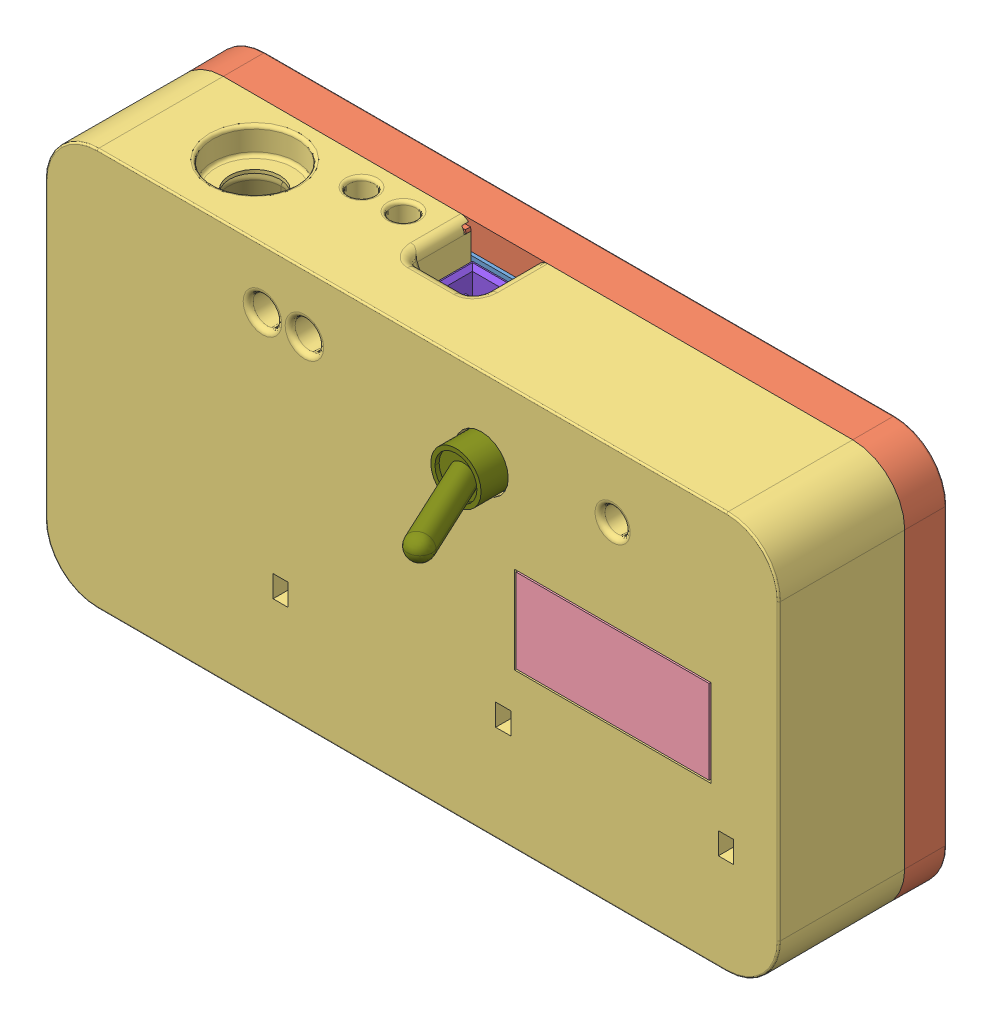
SolidWorks assembly index, configuration 默认. Lengths in mm.
Overall size (87.4 47.4 33.7).
302 component instances, 40 part files, 15 mates.
Components (placement in the parent):
- PowerSupplyBoard-1: PowerSupplyBoard [默认] at origin size (80 40 32.5)
  - PCB2.step-1: PCB2.step [默认] at origin size (80 40 32.5)
    - Board.step-1: Board.step [默认] at origin size (80 40 1.6)
      - Open CASCADE STEP translator 6.8 2.1.1.step-1: Open CASCADE STEP translator 6.8 2.1.1.step [默认] at (0 0 -1.6) size (80 40 1.6)
    - C1.step-1: C1.step [默认] at origin size (0.82 1.6 0.82)
      - C_0603.step-1: C_0603.step [默认] at (74.2189 27.7979 0.0254) x (0 -1 0) z (0 0 1) size (1.6 0.82 0.82)
        - C_0603-7177_AF0_ASM.step-1: C_0603-7177_AF0_ASM.step [默认] at origin size (1.6 0.82 0.82)
          - C_0603-683_AF0_ASM.step-1: C_0603-683_AF0_ASM.step [默认] at origin size (1.6 0.82 0.82)
            - 2_1_200.step-1: 2_1_200.step [默认] at origin size (0.3 0.82 0.82)
            - _1_1_20001.step-1: _1_1_20001.step [默认] at origin size (1 0.8 0.8)
            - 3_1_2_A.step-1: 3_1_2_A.step [默认] at origin size (0.3 0.82 0.82)
    - C3.step-1: C3.step [默认] at origin size (7 6.6 5.41)
      - CM_D(6.3X5.4).step-1: CM_D(6.3X5.4).step [默认] at (74.7014 21.0058 0) x (0 1 0) z (0 0 1) size (6.6 7 5.41)
        - LOGO_.step-1: LOGO_.step [默认] at (1.6383 0.2015 -0.0035) x (-1 0 0) z (0 0 -1) size (1.35 1.56 0.01)
        - CM_D(6.3X5.4)-0.step-1: CM_D(6.3X5.4)-0.step [默认] at origin size (6.6 7 5.41)
    - Open CASCADE STEP translator 6.8 2.4.step-1: Open CASCADE STEP translator 6.8 2.4.step [默认] at origin size (7.54 7.7 9.1)
      - XH2.54-2P_H.step-1: XH2.54-2P_H.step [默认] at (37.2618 32.1564 0.03) x (-1 0 0) z (0 1 0) size (7.54 9.1 7.7)
        - LOGO_-1.step-1: LOGO_-1.step [默认] at (-1.159 -0.003 2.4494) x (0 0 1) z (0 -1 0) size (0.9 1.04 0.01)
        - XH2.54-2P_H-2.step-1: XH2.54-2P_H-2.step [默认] at origin size (7.54 9.1 7.7)
    - Open CASCADE STEP translator 6.8 2.5.step-1: Open CASCADE STEP translator 6.8 2.5.step [默认] at origin size (10.16 12.85 8.1)
      - HDR-1x2_H.step-1: HDR-1x2_H.step [默认] at (40.6527 12.7 0) x (1 0 0) z (0 0 1) size (2.54 12.85 8.1)
        - HDR-1x2_H-3.step-1: HDR-1x2_H-3.step [默认] at origin size (2.54 12.85 8.1)
        - LOGO_-4.step-1: LOGO_-4.step [默认] at (0 -4.7829 0.017) x (-1 0 0) z (0 0 -1) size (0.9 1.04 0.01)
      - HDR-1x2_H.step-2: HDR-1x2_H.step [默认] at (43.1927 12.7 0) x (1 0 0) z (0 0 1) size (2.54 12.85 8.1)
        - HDR-1x2_H-3.step-1: HDR-1x2_H-3.step [默认] at origin size (2.54 12.85 8.1)
        - LOGO_-4.step-1: LOGO_-4.step [默认] at (0 -4.7829 0.017) x (-1 0 0) z (0 0 -1) size (0.9 1.04 0.01)
      - HDR-1x2_H.step-3: HDR-1x2_H.step [默认] at (35.5727 12.7 0) x (1 0 0) z (0 0 1) size (2.54 12.85 8.1)
        - HDR-1x2_H-3.step-1: HDR-1x2_H-3.step [默认] at origin size (2.54 12.85 8.1)
        - LOGO_-4.step-1: LOGO_-4.step [默认] at (0 -4.7829 0.017) x (-1 0 0) z (0 0 -1) size (0.9 1.04 0.01)
      - HDR-1x2_H.step-4: HDR-1x2_H.step [默认] at (38.1127 12.7 0) x (1 0 0) z (0 0 1) size (2.54 12.85 8.1)
        - HDR-1x2_H-3.step-1: HDR-1x2_H-3.step [默认] at origin size (2.54 12.85 8.1)
        - LOGO_-4.step-1: LOGO_-4.step [默认] at (0 -4.7829 0.017) x (-1 0 0) z (0 0 -1) size (0.9 1.04 0.01)
    - Open CASCADE STEP translator 6.8 2.6.step-1: Open CASCADE STEP translator 6.8 2.6.step [默认] at origin size (5 6.01 1.9)
      - SOP8.step-1: SOP8.step [默认] at (39.878 26.6954 0) x (0 1 0) z (0 0 1) size (6.01 5 1.9)
        - LOGO_0.25.step-1: LOGO_0.25.step [默认] at (0.0116 0 0.095) x (0 -1 0) z (0 0 -1) size (0.75 0.87 0.01)
        - SOP8_____.step-1: SOP8_____.step [默认] at origin size (3.6 5 1.8)
        - ____1.8_______.step-1: ____1.8_______.step [默认] at (1.8 1.91 1) x (0 1 0) z (0 0 1) size (0.5 1.2 1.1)
        - ____1.8_______.step-2: ____1.8_______.step [默认] at (1.8 0.64 1) x (0 1 0) z (0 0 1) size (0.5 1.2 1.1)
        - ____1.8_______.step-3: ____1.8_______.step [默认] at (1.8 -0.63 1) x (0 1 0) z (0 0 1) size (0.5 1.2 1.1)
        - ____1.8_______.step-4: ____1.8_______.step [默认] at (1.8 -1.9 1) x (0 1 0) z (0 0 1) size (0.5 1.2 1.1)
        - ____1.8_______.step-5: ____1.8_______.step [默认] at (-1.8 1.91 1) x (0 -1 0) z (0 0 1) size (0.5 1.2 1.1)
        - ____1.8_______.step-6: ____1.8_______.step [默认] at (-1.8 0.64 1) x (0 -1 0) z (0 0 1) size (0.5 1.2 1.1)
        - ____1.8_______.step-7: ____1.8_______.step [默认] at (-1.8 -0.63 1) x (0 -1 0) z (0 0 1) size (0.5 1.2 1.1)
        - ____1.8_______.step-8: ____1.8_______.step [默认] at (-1.8 -1.9 1) x (0 -1 0) z (0 0 1) size (0.5 1.2 1.1)
    - Open CASCADE STEP translator 6.8 2.7.step-1: Open CASCADE STEP translator 6.8 2.7.step [默认] at origin size (5 6.01 1.9)
      - SOP8.step-1: SOP8.step [默认] at (66.9036 26.6954 0) x (0 1 0) z (0 0 1) size (6.01 5 1.9)
        - LOGO_0.25.step-1: LOGO_0.25.step [默认] at (0.0116 0 0.095) x (0 -1 0) z (0 0 -1) size (0.75 0.87 0.01)
        - SOP8_____.step-1: SOP8_____.step [默认] at origin size (3.6 5 1.8)
        - ____1.8_______.step-1: ____1.8_______.step [默认] at (1.8 1.91 1) x (0 1 0) z (0 0 1) size (0.5 1.2 1.1)
        - ____1.8_______.step-2: ____1.8_______.step [默认] at (1.8 0.64 1) x (0 1 0) z (0 0 1) size (0.5 1.2 1.1)
        - ____1.8_______.step-3: ____1.8_______.step [默认] at (1.8 -0.63 1) x (0 1 0) z (0 0 1) size (0.5 1.2 1.1)
        - ____1.8_______.step-4: ____1.8_______.step [默认] at (1.8 -1.9 1) x (0 1 0) z (0 0 1) size (0.5 1.2 1.1)
        - ____1.8_______.step-5: ____1.8_______.step [默认] at (-1.8 1.91 1) x (0 -1 0) z (0 0 1) size (0.5 1.2 1.1)
        - ____1.8_______.step-6: ____1.8_______.step [默认] at (-1.8 0.64 1) x (0 -1 0) z (0 0 1) size (0.5 1.2 1.1)
        - ____1.8_______.step-7: ____1.8_______.step [默认] at (-1.8 -0.63 1) x (0 -1 0) z (0 0 1) size (0.5 1.2 1.1)
        - ____1.8_______.step-8: ____1.8_______.step [默认] at (-1.8 -1.9 1) x (0 -1 0) z (0 0 1) size (0.5 1.2 1.1)
    - R6.step-1: R6.step [默认] at origin size (0.8 1.6 0.4)
      - R0603.step-1: R0603.step [默认] at (44.6277 27.5996 0) x (0 1 0) z (0 0 1) size (1.6 0.8 0.4)
        - R_0603-3615_AF0_ASM.step-1: R_0603-3615_AF0_ASM.step [默认] at origin size (1.6 0.8 0.4)
          - R_0603-3601_AF0_ASM.step-1: R_0603-3601_AF0_ASM.step [默认] at origin size (1.6 0.8 0.4)
            - _2_1_2_3_4_AF0.step-1: _2_1_2_3_4_AF0.step [默认] at origin size (0.25 0.8 0.4)
            - _7_1_2_AF0.step-1: _7_1_2_AF0.step [默认] at origin size (1.5 0.8 0.4)
            - 5_1_2_3_400.step-1: 5_1_2_3_400.step [默认] at origin size (0.25 0.8 0.4)
    - R5.step-1: R5.step [默认] at origin size (0.8 1.6 0.4)
      - R0603.step-1: R0603.step [默认] at (50.8338 12.5832 0) x (0 -1 0) z (0 0 1) size (1.6 0.8 0.4)
        - R_0603-3615_AF0_ASM.step-1: R_0603-3615_AF0_ASM.step [默认] at origin size (1.6 0.8 0.4)
          - R_0603-3601_AF0_ASM.step-1: R_0603-3601_AF0_ASM.step [默认] at origin size (1.6 0.8 0.4)
            - _2_1_2_3_4_AF0.step-1: _2_1_2_3_4_AF0.step [默认] at origin size (0.25 0.8 0.4)
            - _7_1_2_AF0.step-1: _7_1_2_AF0.step [默认] at origin size (1.5 0.8 0.4)
            - 5_1_2_3_400.step-1: 5_1_2_3_400.step [默认] at origin size (0.25 0.8 0.4)
    - R4.step-1: R4.step [默认] at origin size (0.8 1.6 0.4)
      - R0603.step-1: R0603.step [默认] at (47.2185 27.5996 0) x (0 1 0) z (0 0 1) size (1.6 0.8 0.4)
        - R_0603-3615_AF0_ASM.step-1: R_0603-3615_AF0_ASM.step [默认] at origin size (1.6 0.8 0.4)
          - R_0603-3601_AF0_ASM.step-1: R_0603-3601_AF0_ASM.step [默认] at origin size (1.6 0.8 0.4)
            - _2_1_2_3_4_AF0.step-1: _2_1_2_3_4_AF0.step [默认] at origin size (0.25 0.8 0.4)
            - _7_1_2_AF0.step-1: _7_1_2_AF0.step [默认] at origin size (1.5 0.8 0.4)
            - 5_1_2_3_400.step-1: 5_1_2_3_400.step [默认] at origin size (0.25 0.8 0.4)
    - LED2.step-1: LED2.step [默认] at origin size (0.8 1.6 0.61)
      - LED_0603-G(1).step-1: LED_0603-G(1).step [默认] at (50.8649 9.0649 0) x (0 1 0) z (0 0 1) size (1.6 0.8 0.47)
        - LED_0603-G-7058_AF0_ASM.step-1: LED_0603-G-7058_AF0_ASM.step [默认] at origin size (1.6 0.8 0.47)
          - LED_0603-G-4339_AF0_ASM.step-1: LED_0603-G-4339_AF0_ASM.step [默认] at origin size (1.6 0.8 0.47)
            - 4_100.step-1: 4_100.step [默认] at origin size (0.2 0.8 0.2)
            - _2_10001.step-1: _2_10001.step [默认] at origin size (0.2 0.8 0.2)
            - _5_2__10001.step-1: _5_2__10001.step [默认] at origin size (0.31 0.14 0)
            - _5_1__10001.step-1: _5_1__10001.step [默认] at origin size (0.31 0.14 0)
            - 1_1_2_3_4_5_6_7_8_0.step-1: 1_1_2_3_4_5_6_7_8_0.step [默认] at origin size (1.6 0.8 0.47)
      - LED_0603______.step-1: LED_0603______.step [默认] at (50.8649 9.0649 0) x (0 -1 0) z (0 0 1) size (1.2 0.8 0.4)
    - Open CASCADE STEP translator 6.8 2.12.step-1: Open CASCADE STEP translator 6.8 2.12.step [默认] at origin size (6.95 6.6 3.03)
      - SMD-0630.step-1: SMD-0630.step [默认] at (39.4682 18.3134 0) x (1 0 0) z (0 0 1) size (6.95 6.6 3.03)
        - SMD-0630-5.step-1: SMD-0630-5.step [默认] at origin size (6.95 6.6 3.03)
        - LOGO_0.5.step-1: LOGO_0.5.step [默认] at (0 0.0017 0.04) size (1.5 1.73 0.01)
    - F2.step-1: F2.step [默认] at origin size (3.22 4.6 0.87)
      - FU_01812.step-1: FU_01812.step [默认] at (47.0662 11.7496 0) x (0 -1 0) z (0 0 1) size (4.6 3.22 0.87)
        - LOGO_-6.step-1: LOGO_-6.step [默认] at (0 0.0363 0.009) x (-1 0 0) z (0 0 -1) size (0.6 0.69 0)
        - FU_1812.step-1: FU_1812.step [默认] at origin size (4.6 3.22 0.87)
    - D2.step-1: D2.step [默认] at origin size (2.6 5.12 2.1)
      - SMA.step-1: SMA.step [默认] at (31.2327 15.471 0.0508) x (0 1 0) z (0 0 1) size (5.12 2.6 2.1)
        - SMA-4715_AF0_ASM.step-1: SMA-4715_AF0_ASM.step [默认] at origin size (5.12 2.6 2.1)
          - SMA-5401_AF0.step-1: SMA-5401_AF0.step [默认] at origin size (5.12 2.6 2.1)
    - C12.step-1: C12.step [默认] at origin size (0.82 1.6 0.82)
      - C_0603.step-1: C_0603.step [默认] at (6.9851 16.7489 0.0254) x (0 -1 0) z (0 0 1) size (1.6 0.82 0.82)
        - C_0603-7177_AF0_ASM.step-1: C_0603-7177_AF0_ASM.step [默认] at origin size (1.6 0.82 0.82)
          - C_0603-683_AF0_ASM.step-1: C_0603-683_AF0_ASM.step [默认] at origin size (1.6 0.82 0.82)
            - 2_1_200.step-1: 2_1_200.step [默认] at origin size (0.3 0.82 0.82)
            - _1_1_20001.step-1: _1_1_20001.step [默认] at origin size (1 0.8 0.8)
            - 3_1_2_A.step-1: 3_1_2_A.step [默认] at origin size (0.3 0.82 0.82)
    - C10.step-1: C10.step [默认] at origin size (0.82 1.6 0.82)
      - C_0603.step-1: C_0603.step [默认] at (19.8248 16.7489 0.0254) x (0 -1 0) z (0 0 1) size (1.6 0.82 0.82)
        - C_0603-7177_AF0_ASM.step-1: C_0603-7177_AF0_ASM.step [默认] at origin size (1.6 0.82 0.82)
          - C_0603-683_AF0_ASM.step-1: C_0603-683_AF0_ASM.step [默认] at origin size (1.6 0.82 0.82)
            - 2_1_200.step-1: 2_1_200.step [默认] at origin size (0.3 0.82 0.82)
            - _1_1_20001.step-1: _1_1_20001.step [默认] at origin size (1 0.8 0.8)
            - 3_1_2_A.step-1: 3_1_2_A.step [默认] at origin size (0.3 0.82 0.82)
    - C9.step-1: C9.step [默认] at origin size (1.6 0.82 0.82)
      - C_0603.step-1: C_0603.step [默认] at (49.7689 16.1289 0.0254) x (-1 0 0) z (0 0 1) size (1.6 0.82 0.82)
        - C_0603-7177_AF0_ASM.step-1: C_0603-7177_AF0_ASM.step [默认] at origin size (1.6 0.82 0.82)
          - C_0603-683_AF0_ASM.step-1: C_0603-683_AF0_ASM.step [默认] at origin size (1.6 0.82 0.82)
            - 2_1_200.step-1: 2_1_200.step [默认] at origin size (0.3 0.82 0.82)
            - _1_1_20001.step-1: _1_1_20001.step [默认] at origin size (1 0.8 0.8)
            - 3_1_2_A.step-1: 3_1_2_A.step [默认] at origin size (0.3 0.82 0.82)
    - C8.step-1: C8.step [默认] at origin size (0.82 1.6 0.82)
      - C_0603.step-1: C_0603.step [默认] at (35.9681 25.8961 0.0254) x (0 -1 0) z (0 0 1) size (1.6 0.82 0.82)
        - C_0603-7177_AF0_ASM.step-1: C_0603-7177_AF0_ASM.step [默认] at origin size (1.6 0.82 0.82)
          - C_0603-683_AF0_ASM.step-1: C_0603-683_AF0_ASM.step [默认] at origin size (1.6 0.82 0.82)
            - 2_1_200.step-1: 2_1_200.step [默认] at origin size (0.3 0.82 0.82)
            - _1_1_20001.step-1: _1_1_20001.step [默认] at origin size (1 0.8 0.8)
            - 3_1_2_A.step-1: 3_1_2_A.step [默认] at origin size (0.3 0.82 0.82)
    - C7.step-1: C7.step [默认] at origin size (7 6.6 5.41)
      - CM_D(6.3X5.4).step-1: CM_D(6.3X5.4).step [默认] at (49.4284 21.0058 0) x (0 1 0) z (0 0 1) size (6.6 7 5.41)
        - LOGO_.step-1: LOGO_.step [默认] at (1.6383 0.2015 -0.0035) x (-1 0 0) z (0 0 -1) size (1.35 1.56 0.01)
        - CM_D(6.3X5.4)-0.step-1: CM_D(6.3X5.4)-0.step [默认] at origin size (6.6 7 5.41)
    - C6.step-1: C6.step [默认] at origin size (6.6 7 5.41)
      - CM_D(6.3X5.4).step-1: CM_D(6.3X5.4).step [默认] at (31.242 25.8318 0) x (-1 0 0) z (0 0 1) size (6.6 7 5.41)
        - LOGO_.step-1: LOGO_.step [默认] at (1.6383 0.2015 -0.0035) x (-1 0 0) z (0 0 -1) size (1.35 1.56 0.01)
        - CM_D(6.3X5.4)-0.step-1: CM_D(6.3X5.4)-0.step [默认] at origin size (6.6 7 5.41)
    - C13.step-1: C13.step [默认] at origin size (0.82 1.6 0.82)
      - C_0603.step-1: C_0603.step [默认] at (5.2071 16.7489 0.0254) x (0 -1 0) z (0 0 1) size (1.6 0.82 0.82)
        - C_0603-7177_AF0_ASM.step-1: C_0603-7177_AF0_ASM.step [默认] at origin size (1.6 0.82 0.82)
          - C_0603-683_AF0_ASM.step-1: C_0603-683_AF0_ASM.step [默认] at origin size (1.6 0.82 0.82)
            - 2_1_200.step-1: 2_1_200.step [默认] at origin size (0.3 0.82 0.82)
            - _1_1_20001.step-1: _1_1_20001.step [默认] at origin size (1 0.8 0.8)
            - 3_1_2_A.step-1: 3_1_2_A.step [默认] at origin size (0.3 0.82 0.82)
    - Open CASCADE STEP translator 6.8 2.22.step-1: Open CASCADE STEP translator 6.8 2.22.step [默认] at origin size (10.5 7.6 13.8)
      - KF301.step-1: KF301.step [默认] at (27.1742 36.6776 0.05) x (-1 0 0) z (0 0 1) size (5.5 7.6 13.8)
        - LOGO_-7.step-1: LOGO_-7.step [默认] at (0 1.4435 -0.0028) x (-1 0 0) z (0 0 -1) size (0.84 0.97 0.01)
        - KF301-8.step-1: KF301-8.step [默认] x (1 0 0) z (0 -1 0) size (5.5 13.8 7.6)
      - KF301.step-2: KF301.step [默认] at (22.1742 36.6776 0.05) x (-1 0 0) z (0 0 1) size (5.5 7.6 13.8)
        - LOGO_-7.step-1: LOGO_-7.step [默认] at (0 1.4435 -0.0028) x (-1 0 0) z (0 0 -1) size (0.84 0.97 0.01)
        - KF301-8.step-1: KF301-8.step [默认] x (1 0 0) z (0 -1 0) size (5.5 13.8 7.6)
    - Open CASCADE STEP translator 6.8 2.23.step-1: Open CASCADE STEP translator 6.8 2.23.step [默认] at origin size (9.3 14.05 15)
      - dc-005.step-1: dc-005.step [默认] at (12.9532 32.2582 0.2) x (-1 0 0) z (0 0 1) size (9.3 14.05 15)
    - C5.step-1: C5.step [默认] at origin size (1.6 0.82 0.82)
      - C_0603.step-1: C_0603.step [默认] at (75.2197 16.1289 0.0254) x (-1 0 0) z (0 0 1) size (1.6 0.82 0.82)
        - C_0603-7177_AF0_ASM.step-1: C_0603-7177_AF0_ASM.step [默认] at origin size (1.6 0.82 0.82)
          - C_0603-683_AF0_ASM.step-1: C_0603-683_AF0_ASM.step [默认] at origin size (1.6 0.82 0.82)
            - 2_1_200.step-1: 2_1_200.step [默认] at origin size (0.3 0.82 0.82)
            - _1_1_20001.step-1: _1_1_20001.step [默认] at origin size (1 0.8 0.8)
            - 3_1_2_A.step-1: 3_1_2_A.step [默认] at origin size (0.3 0.82 0.82)
    - Open CASCADE STEP translator 6.8 2.25.step-1: Open CASCADE STEP translator 6.8 2.25.step [默认] at origin size (6.51 7.02 1.67)
      - SOT223.step-1: SOT223.step [默认] at (12.6231 19.5037 0) x (1 0 0) z (0 0 1) size (6.51 7.02 1.67)
        - SOT223-4091_AF0_ASM.step-1: SOT223-4091_AF0_ASM.step [默认] at origin size (6.51 7.02 1.67)
          - SOT223_-20.step-1: SOT223_-20.step [默认] at (-2.3 -1.75 0.725) x (-1 0 0) z (0 0 1) size (0.71 1.76 0.92)
          - SOT223-16115_AF0.step-1: SOT223-16115_AF0.step [默认] at origin size (6.51 3.51 1.6)
          - SOT223_-10.step-1: SOT223_-10.step [默认] at (0 1.75 0.725) size (3 1.76 0.92)
          - SOT223_-20.step-2: SOT223_-20.step [默认] at (2.3 -1.75 0.725) x (-1 0 0) z (0 0 1) size (0.71 1.76 0.92)
          - SOT223_-20.step-3: SOT223_-20.step [默认] at (0 -1.75 0.725) x (-1 0 0) z (0 0 1) size (0.71 1.76 0.92)
    - S1.step-1: S1.step [默认] at origin size (12.72 10.16 32.39)
      - User_Library-7101SYZQE_switch-toggle.step-1: User_Library-7101SYZQE_switch-toggle.step [默认] at (48.26 34.2138 9.144) x (0 0 -1) z (1 0 0) size (32.39 10.16 12.72)
    - R9.step-1: R9.step [默认] at origin size (0.8 1.6 0.4)
      - R0603.step-1: R0603.step [默认] at (57.5666 36.0794 0) x (0 -1 0) z (0 0 1) size (1.6 0.8 0.4)
        - R_0603-3615_AF0_ASM.step-1: R_0603-3615_AF0_ASM.step [默认] at origin size (1.6 0.8 0.4)
          - R_0603-3601_AF0_ASM.step-1: R_0603-3601_AF0_ASM.step [默认] at origin size (1.6 0.8 0.4)
            - _2_1_2_3_4_AF0.step-1: _2_1_2_3_4_AF0.step [默认] at origin size (0.25 0.8 0.4)
            - _7_1_2_AF0.step-1: _7_1_2_AF0.step [默认] at origin size (1.5 0.8 0.4)
            - 5_1_2_3_400.step-1: 5_1_2_3_400.step [默认] at origin size (0.25 0.8 0.4)
    - R8.step-1: R8.step [默认] at origin size (0.8 1.6 0.4)
      - R0603.step-1: R0603.step [默认] at (21.9965 16.7234 0) x (0 -1 0) z (0 0 1) size (1.6 0.8 0.4)
        - R_0603-3615_AF0_ASM.step-1: R_0603-3615_AF0_ASM.step [默认] at origin size (1.6 0.8 0.4)
          - R_0603-3601_AF0_ASM.step-1: R_0603-3601_AF0_ASM.step [默认] at origin size (1.6 0.8 0.4)
            - _2_1_2_3_4_AF0.step-1: _2_1_2_3_4_AF0.step [默认] at origin size (0.25 0.8 0.4)
            - _7_1_2_AF0.step-1: _7_1_2_AF0.step [默认] at origin size (1.5 0.8 0.4)
            - 5_1_2_3_400.step-1: 5_1_2_3_400.step [默认] at origin size (0.25 0.8 0.4)
    - R7.step-1: R7.step [默认] at origin size (0.8 1.6 0.4)
      - R0603.step-1: R0603.step [默认] at (24.2991 12.5832 0) x (0 -1 0) z (0 0 1) size (1.6 0.8 0.4)
        - R_0603-3615_AF0_ASM.step-1: R_0603-3615_AF0_ASM.step [默认] at origin size (1.6 0.8 0.4)
          - R_0603-3601_AF0_ASM.step-1: R_0603-3601_AF0_ASM.step [默认] at origin size (1.6 0.8 0.4)
            - _2_1_2_3_4_AF0.step-1: _2_1_2_3_4_AF0.step [默认] at origin size (0.25 0.8 0.4)
            - _7_1_2_AF0.step-1: _7_1_2_AF0.step [默认] at origin size (1.5 0.8 0.4)
            - 5_1_2_3_400.step-1: 5_1_2_3_400.step [默认] at origin size (0.25 0.8 0.4)
    - R3.step-1: R3.step [默认] at origin size (0.8 1.6 0.4)
      - R0603.step-1: R0603.step [默认] at (77.3685 12.5832 0) x (0 -1 0) z (0 0 1) size (1.6 0.8 0.4)
        - R_0603-3615_AF0_ASM.step-1: R_0603-3615_AF0_ASM.step [默认] at origin size (1.6 0.8 0.4)
          - R_0603-3601_AF0_ASM.step-1: R_0603-3601_AF0_ASM.step [默认] at origin size (1.6 0.8 0.4)
            - _2_1_2_3_4_AF0.step-1: _2_1_2_3_4_AF0.step [默认] at origin size (0.25 0.8 0.4)
            - _7_1_2_AF0.step-1: _7_1_2_AF0.step [默认] at origin size (1.5 0.8 0.4)
            - 5_1_2_3_400.step-1: 5_1_2_3_400.step [默认] at origin size (0.25 0.8 0.4)
    - R2.step-1: R2.step [默认] at origin size (9.5 4.8 15)
      - 3296.step-1: 3296.step [默认] at (67.4409 34.6711 0.02) x (-1 0 0) z (0 0 1) size (9.5 4.8 15)
        - 3296-10.step-1: 3296-10.step [默认] at origin size (9.5 4.8 15)
        - LOGO_-11.step-1: LOGO_-11.step [默认] at (1.2121 -0.8676 0.494) x (-1 0 0) z (0 0 -1) size (1.8 2.08 0.01)
    - R1.step-1: R1.step [默认] at origin size (0.8 1.6 0.4)
      - R0603.step-1: R0603.step [默认] at (71.6533 27.5996 0) x (0 1 0) z (0 0 1) size (1.6 0.8 0.4)
        - R_0603-3615_AF0_ASM.step-1: R_0603-3615_AF0_ASM.step [默认] at origin size (1.6 0.8 0.4)
          - R_0603-3601_AF0_ASM.step-1: R_0603-3601_AF0_ASM.step [默认] at origin size (1.6 0.8 0.4)
            - _2_1_2_3_4_AF0.step-1: _2_1_2_3_4_AF0.step [默认] at origin size (0.25 0.8 0.4)
            - _7_1_2_AF0.step-1: _7_1_2_AF0.step [默认] at origin size (1.5 0.8 0.4)
            - 5_1_2_3_400.step-1: 5_1_2_3_400.step [默认] at origin size (0.25 0.8 0.4)
    - Q1.step-1: Q1.step [默认] at origin size (6.73 10.1 2.4)
      - DPAK_TO-252AA.step-1: DPAK_TO-252AA.step [默认] at (22.5553 26.1736 0.127) x (1 0 0) z (0 -1 0) size (6.73 2.4 10.1)
    - LED4.step-1: LED4.step [默认] at origin size (0.8 1.6 0.61)
      - LED_0603-G(1).step-1: LED_0603-G(1).step [默认] at (59.7183 35.8962 0) x (0 1 0) z (0 0 1) size (1.6 0.8 0.47)
        - LED_0603-G-7058_AF0_ASM.step-1: LED_0603-G-7058_AF0_ASM.step [默认] at origin size (1.6 0.8 0.47)
          - LED_0603-G-4339_AF0_ASM.step-1: LED_0603-G-4339_AF0_ASM.step [默认] at origin size (1.6 0.8 0.47)
            - 4_100.step-1: 4_100.step [默认] at origin size (0.2 0.8 0.2)
            - _2_10001.step-1: _2_10001.step [默认] at origin size (0.2 0.8 0.2)
            - _5_2__10001.step-1: _5_2__10001.step [默认] at origin size (0.31 0.14 0)
            - _5_1__10001.step-1: _5_1__10001.step [默认] at origin size (0.31 0.14 0)
            - 1_1_2_3_4_5_6_7_8_0.step-1: 1_1_2_3_4_5_6_7_8_0.step [默认] at origin size (1.6 0.8 0.47)
      - LED_0603______.step-1: LED_0603______.step [默认] at (59.7183 35.8962 0) x (0 -1 0) z (0 0 1) size (1.2 0.8 0.4)
    - LED3.step-1: LED3.step [默认] at origin size (0.8 1.6 0.61)
      - LED_0603-G(1).step-1: LED_0603-G(1).step [默认] at (24.3395 9.0649 0) x (0 1 0) z (0 0 1) size (1.6 0.8 0.47)
        - LED_0603-G-7058_AF0_ASM.step-1: LED_0603-G-7058_AF0_ASM.step [默认] at origin size (1.6 0.8 0.47)
          - LED_0603-G-4339_AF0_ASM.step-1: LED_0603-G-4339_AF0_ASM.step [默认] at origin size (1.6 0.8 0.47)
            - 4_100.step-1: 4_100.step [默认] at origin size (0.2 0.8 0.2)
            - _2_10001.step-1: _2_10001.step [默认] at origin size (0.2 0.8 0.2)
            - _5_2__10001.step-1: _5_2__10001.step [默认] at origin size (0.31 0.14 0)
            - _5_1__10001.step-1: _5_1__10001.step [默认] at origin size (0.31 0.14 0)
            - 1_1_2_3_4_5_6_7_8_0.step-1: 1_1_2_3_4_5_6_7_8_0.step [默认] at origin size (1.6 0.8 0.47)
      - LED_0603______.step-1: LED_0603______.step [默认] at (24.3395 9.0649 0) x (0 -1 0) z (0 0 1) size (1.2 0.8 0.4)
    - LED1.step-1: LED1.step [默认] at origin size (0.8 1.6 0.61)
      - LED_0603-G(1).step-1: LED_0603-G(1).step [默认] at (77.3902 9.0649 0) x (0 1 0) z (0 0 1) size (1.6 0.8 0.47)
        - LED_0603-G-7058_AF0_ASM.step-1: LED_0603-G-7058_AF0_ASM.step [默认] at origin size (1.6 0.8 0.47)
          - LED_0603-G-4339_AF0_ASM.step-1: LED_0603-G-4339_AF0_ASM.step [默认] at origin size (1.6 0.8 0.47)
            - 4_100.step-1: 4_100.step [默认] at origin size (0.2 0.8 0.2)
            - _2_10001.step-1: _2_10001.step [默认] at origin size (0.2 0.8 0.2)
            - _5_2__10001.step-1: _5_2__10001.step [默认] at origin size (0.31 0.14 0)
            - _5_1__10001.step-1: _5_1__10001.step [默认] at origin size (0.31 0.14 0)
            - 1_1_2_3_4_5_6_7_8_0.step-1: 1_1_2_3_4_5_6_7_8_0.step [默认] at origin size (1.6 0.8 0.47)
      - LED_0603______.step-1: LED_0603______.step [默认] at (77.3902 9.0649 0) x (0 -1 0) z (0 0 1) size (1.2 0.8 0.4)
    - Open CASCADE STEP translator 6.8 2.37.step-1: Open CASCADE STEP translator 6.8 2.37.step [默认] at origin size (6.95 6.6 3.03)
      - SMD-0630.step-1: SMD-0630.step [默认] at (65.808 18.3134 0) x (1 0 0) z (0 0 1) size (6.95 6.6 3.03)
        - SMD-0630-5.step-1: SMD-0630-5.step [默认] at origin size (6.95 6.6 3.03)
        - LOGO_0.5.step-1: LOGO_0.5.step [默认] at (0 0.0017 0.04) size (1.5 1.73 0.01)
    - Open CASCADE STEP translator 6.8 2.38.step-1: Open CASCADE STEP translator 6.8 2.38.step [默认] at origin size (10.16 12.85 8.1)
      - HDR-1x2_H.step-1: HDR-1x2_H.step [默认] at (14.224 12.7 0) x (1 0 0) z (0 0 1) size (2.54 12.85 8.1)
        - HDR-1x2_H-3.step-1: HDR-1x2_H-3.step [默认] at origin size (2.54 12.85 8.1)
        - LOGO_-4.step-1: LOGO_-4.step [默认] at (0 -4.7829 0.017) x (-1 0 0) z (0 0 -1) size (0.9 1.04 0.01)
      - HDR-1x2_H.step-2: HDR-1x2_H.step [默认] at (16.764 12.7 0) x (1 0 0) z (0 0 1) size (2.54 12.85 8.1)
        - HDR-1x2_H-3.step-1: HDR-1x2_H-3.step [默认] at origin size (2.54 12.85 8.1)
        - LOGO_-4.step-1: LOGO_-4.step [默认] at (0 -4.7829 0.017) x (-1 0 0) z (0 0 -1) size (0.9 1.04 0.01)
      - HDR-1x2_H.step-3: HDR-1x2_H.step [默认] at (9.144 12.7 0) x (1 0 0) z (0 0 1) size (2.54 12.85 8.1)
        - HDR-1x2_H-3.step-1: HDR-1x2_H-3.step [默认] at origin size (2.54 12.85 8.1)
        - LOGO_-4.step-1: LOGO_-4.step [默认] at (0 -4.7829 0.017) x (-1 0 0) z (0 0 -1) size (0.9 1.04 0.01)
      - HDR-1x2_H.step-4: HDR-1x2_H.step [默认] at (11.684 12.7 0) x (1 0 0) z (0 0 1) size (2.54 12.85 8.1)
        - HDR-1x2_H-3.step-1: HDR-1x2_H-3.step [默认] at origin size (2.54 12.85 8.1)
        - LOGO_-4.step-1: LOGO_-4.step [默认] at (0 -4.7829 0.017) x (-1 0 0) z (0 0 -1) size (0.9 1.04 0.01)
    - Open CASCADE STEP translator 6.8 2.39.step-1: Open CASCADE STEP translator 6.8 2.39.step [默认] at origin size (10.16 12.85 8.1)
      - HDR-1x2_H.step-1: HDR-1x2_H.step [默认] at (67.0814 12.7 0) x (1 0 0) z (0 0 1) size (2.54 12.85 8.1)
        - HDR-1x2_H-3.step-1: HDR-1x2_H-3.step [默认] at origin size (2.54 12.85 8.1)
        - LOGO_-4.step-1: LOGO_-4.step [默认] at (0 -4.7829 0.017) x (-1 0 0) z (0 0 -1) size (0.9 1.04 0.01)
      - HDR-1x2_H.step-2: HDR-1x2_H.step [默认] at (69.6214 12.7 0) x (1 0 0) z (0 0 1) size (2.54 12.85 8.1)
        - HDR-1x2_H-3.step-1: HDR-1x2_H-3.step [默认] at origin size (2.54 12.85 8.1)
        - LOGO_-4.step-1: LOGO_-4.step [默认] at (0 -4.7829 0.017) x (-1 0 0) z (0 0 -1) size (0.9 1.04 0.01)
      - HDR-1x2_H.step-3: HDR-1x2_H.step [默认] at (62.0014 12.7 0) x (1 0 0) z (0 0 1) size (2.54 12.85 8.1)
        - HDR-1x2_H-3.step-1: HDR-1x2_H-3.step [默认] at origin size (2.54 12.85 8.1)
        - LOGO_-4.step-1: LOGO_-4.step [默认] at (0 -4.7829 0.017) x (-1 0 0) z (0 0 -1) size (0.9 1.04 0.01)
      - HDR-1x2_H.step-4: HDR-1x2_H.step [默认] at (64.5414 12.7 0) x (1 0 0) z (0 0 1) size (2.54 12.85 8.1)
        - HDR-1x2_H-3.step-1: HDR-1x2_H-3.step [默认] at origin size (2.54 12.85 8.1)
        - LOGO_-4.step-1: LOGO_-4.step [默认] at (0 -4.7829 0.017) x (-1 0 0) z (0 0 -1) size (0.9 1.04 0.01)
    - F3.step-1: F3.step [默认] at origin size (3.22 4.6 0.87)
      - FU_01812.step-1: FU_01812.step [默认] at (20.5994 11.7496 0) x (0 -1 0) z (0 0 1) size (4.6 3.22 0.87)
        - LOGO_-6.step-1: LOGO_-6.step [默认] at (0 0.0363 0.009) x (-1 0 0) z (0 0 -1) size (0.6 0.69 0)
        - FU_1812.step-1: FU_1812.step [默认] at origin size (4.6 3.22 0.87)
    - F1.step-1: F1.step [默认] at origin size (3.22 4.6 0.87)
      - FU_01812.step-1: FU_01812.step [默认] at (73.533 11.7496 0) x (0 -1 0) z (0 0 1) size (4.6 3.22 0.87)
        - LOGO_-6.step-1: LOGO_-6.step [默认] at (0 0.0363 0.009) x (-1 0 0) z (0 0 -1) size (0.6 0.69 0)
        - FU_1812.step-1: FU_1812.step [默认] at origin size (4.6 3.22 0.87)
    - D1.step-1: D1.step [默认] at origin size (2.6 5.12 2.1)
      - SMA.step-1: SMA.step [默认] at (58.1567 15.471 0.0508) x (0 1 0) z (0 0 1) size (5.12 2.6 2.1)
        - SMA-4715_AF0_ASM.step-1: SMA-4715_AF0_ASM.step [默认] at origin size (5.12 2.6 2.1)
          - SMA-5401_AF0.step-1: SMA-5401_AF0.step [默认] at origin size (5.12 2.6 2.1)
    - C11.step-1: C11.step [默认] at origin size (0.82 1.6 0.82)
      - C_0603.step-1: C_0603.step [默认] at (17.7039 16.7489 0.0254) x (0 -1 0) z (0 0 1) size (1.6 0.82 0.82)
        - C_0603-7177_AF0_ASM.step-1: C_0603-7177_AF0_ASM.step [默认] at origin size (1.6 0.82 0.82)
          - C_0603-683_AF0_ASM.step-1: C_0603-683_AF0_ASM.step [默认] at origin size (1.6 0.82 0.82)
            - 2_1_200.step-1: 2_1_200.step [默认] at origin size (0.3 0.82 0.82)
            - _1_1_20001.step-1: _1_1_20001.step [默认] at origin size (1 0.8 0.8)
            - 3_1_2_A.step-1: 3_1_2_A.step [默认] at origin size (0.3 0.82 0.82)
    - C4.step-1: C4.step [默认] at origin size (0.82 1.6 0.82)
      - C_0603.step-1: C_0603.step [默认] at (63.0175 25.8961 0.0254) x (0 -1 0) z (0 0 1) size (1.6 0.82 0.82)
        - C_0603-7177_AF0_ASM.step-1: C_0603-7177_AF0_ASM.step [默认] at origin size (1.6 0.82 0.82)
          - C_0603-683_AF0_ASM.step-1: C_0603-683_AF0_ASM.step [默认] at origin size (1.6 0.82 0.82)
            - 2_1_200.step-1: 2_1_200.step [默认] at origin size (0.3 0.82 0.82)
            - _1_1_20001.step-1: _1_1_20001.step [默认] at origin size (1 0.8 0.8)
            - 3_1_2_A.step-1: 3_1_2_A.step [默认] at origin size (0.3 0.82 0.82)
    - C2.step-1: C2.step [默认] at origin size (6.6 7 5.41)
      - CM_D(6.3X5.4).step-1: CM_D(6.3X5.4).step [默认] at (58.2676 25.8318 0) x (-1 0 0) z (0 0 1) size (6.6 7 5.41)
        - LOGO_.step-1: LOGO_.step [默认] at (1.6383 0.2015 -0.0035) x (-1 0 0) z (0 0 -1) size (1.35 1.56 0.01)
        - CM_D(6.3X5.4)-0.step-1: CM_D(6.3X5.4)-0.step [默认] at origin size (6.6 7 5.41)
- ShellBottom-1: ShellBottom [默认] at (0 0 -1.6) x (-1 0 0) z (0 0 -1) size (87.4 47.4 5.6)
- ShellTop-1: ShellTop [默认] at origin size (87.4 47.4 15)
- Voltmeter-1: Voltmeter [默认] at (63.8909 20 7.6) size (30 11 9)
Mates (geometry in assembly coordinates):
- 重合1: coincident aligned: plane of PowerSupplyBoard-1 through (0 0 0) normal (0 0 1)
- 重合2: coincident aligned: plane of PowerSupplyBoard-1 through (0 0 0) normal (0 1 0)
- 重合3: coincident aligned: plane of PowerSupplyBoard-1 through (0 0 0) normal (1 0 0)
- 在位1: in place: plane of PowerSupplyBoard-1/PCB2.step-1/Board.step-1/Open CASCADE STEP translator 6.8 2.1.1.step-1 through (0 2.5 -1.6) normal (0 0 -1); plane of ShellBottom-1 through (0 0 -1.6) normal (0 0 -1); moOrthogonalPlaneRef_w of PowerSupplyBoard-1/PCB2.step-1/Board.step-1/Open CASCADE STEP translator 6.8 2.1.1.step-1 through (0 2.5 -1.6) normal (0 0 -1); plane of ShellBottom-1 through (0 0 -1.6) normal (0 1 0); plane of PowerSupplyBoard-1/PCB2.step-1/Board.step-1/Open CASCADE STEP translator 6.8 2.1.1.step-1 through (0 2.5 -1.6) normal (0 0 -1); plane of ShellBottom-1 through (0 0 -1.6) normal (-1 0 0); plane of PowerSupplyBoard-1/PCB2.step-1/Board.step-1/Open CASCADE STEP translator 6.8 2.1.1.step-1 through (0 2.5 -1.6) normal (0 0 -1); unknown of ShellBottom-1
- 重合4: coincident aligned: plane of PowerSupplyBoard-1/PCB2.step-1/Board.step-1/Open CASCADE STEP translator 6.8 2.1.1.step-1; plane of ShellBottom-1
- 重合5: coincident aligned: moOrthogonalPlaneRef_w of PowerSupplyBoard-1/PCB2.step-1/Board.step-1/Open CASCADE STEP translator 6.8 2.1.1.step-1 through (0 0 -1.6) normal (0 1 0); plane of ShellBottom-1 through (0 0 -1.6) normal (0 1 0)
- 重合6: coincident anti-aligned: moOrthogonalPlaneRef_w of PowerSupplyBoard-1/PCB2.step-1/Board.step-1/Open CASCADE STEP translator 6.8 2.1.1.step-1 through (0 0 -1.6) normal (1 0 0); plane of ShellBottom-1 through (0 0 -1.6) normal (-1 0 0)
- 在位2: in place: plane of PowerSupplyBoard-1/PCB2.step-1/Board.step-1/Open CASCADE STEP translator 6.8 2.1.1.step-1 through (0 2.5 0) normal (0 0 1); plane of ShellTop-1 through (0 0 0) normal (0 0 1); plane of PowerSupplyBoard-1/PCB2.step-1/Board.step-1/Open CASCADE STEP translator 6.8 2.1.1.step-1 through (0 2.5 0) normal (0 0 1); plane of ShellTop-1 through (0 0 0) normal (0 1 0); plane of PowerSupplyBoard-1/PCB2.step-1/Board.step-1/Open CASCADE STEP translator 6.8 2.1.1.step-1 through (0 2.5 0) normal (0 0 1); plane of ShellTop-1 through (0 0 0) normal (1 0 0); plane of PowerSupplyBoard-1/PCB2.step-1/Board.step-1/Open CASCADE STEP translator 6.8 2.1.1.step-1 through (0 2.5 0) normal (0 0 1); unknown of ShellTop-1
- 重合4: coincident aligned: plane of PowerSupplyBoard-1/PCB2.step-1/Board.step-1/Open CASCADE STEP translator 6.8 2.1.1.step-1; plane of ShellTop-1
- 重合5: coincident aligned: moOrthogonalPlaneRef_w of PowerSupplyBoard-1/PCB2.step-1/Board.step-1/Open CASCADE STEP translator 6.8 2.1.1.step-1 through (0 0 0) normal (0 1 0); plane of ShellTop-1 through (0 0 0) normal (0 1 0)
- 重合6: coincident anti-aligned: moOrthogonalPlaneRef_w of PowerSupplyBoard-1/PCB2.step-1/Board.step-1/Open CASCADE STEP translator 6.8 2.1.1.step-1 through (0 0 0) normal (-1 0 0); plane of ShellTop-1 through (0 0 0) normal (1 0 0)
- 重合4: coincident: line of ShellTop-1 through (63.8909 35.8711 10.82) axis (0 0 1); plane of Voltmeter-1 through (63.8909 20 7.6) normal (1 0 0)
- 平行1: parallel aligned: plane of ShellTop-1 through (0 0 0) normal (0 1 0); plane of Voltmeter-1 through (63.8909 20 7.6) normal (0 1 0)
- 重合6: coincident aligned: plane of ShellTop-1 through (2.4992 37.5008 15) normal (0 0 1); plane of Voltmeter-1 through (63.8909 20 15) normal (0 0 1)
- 重合7: coincident aligned: plane of Voltmeter-1 through (63.8909 20 7.6) normal (0 1 0)
